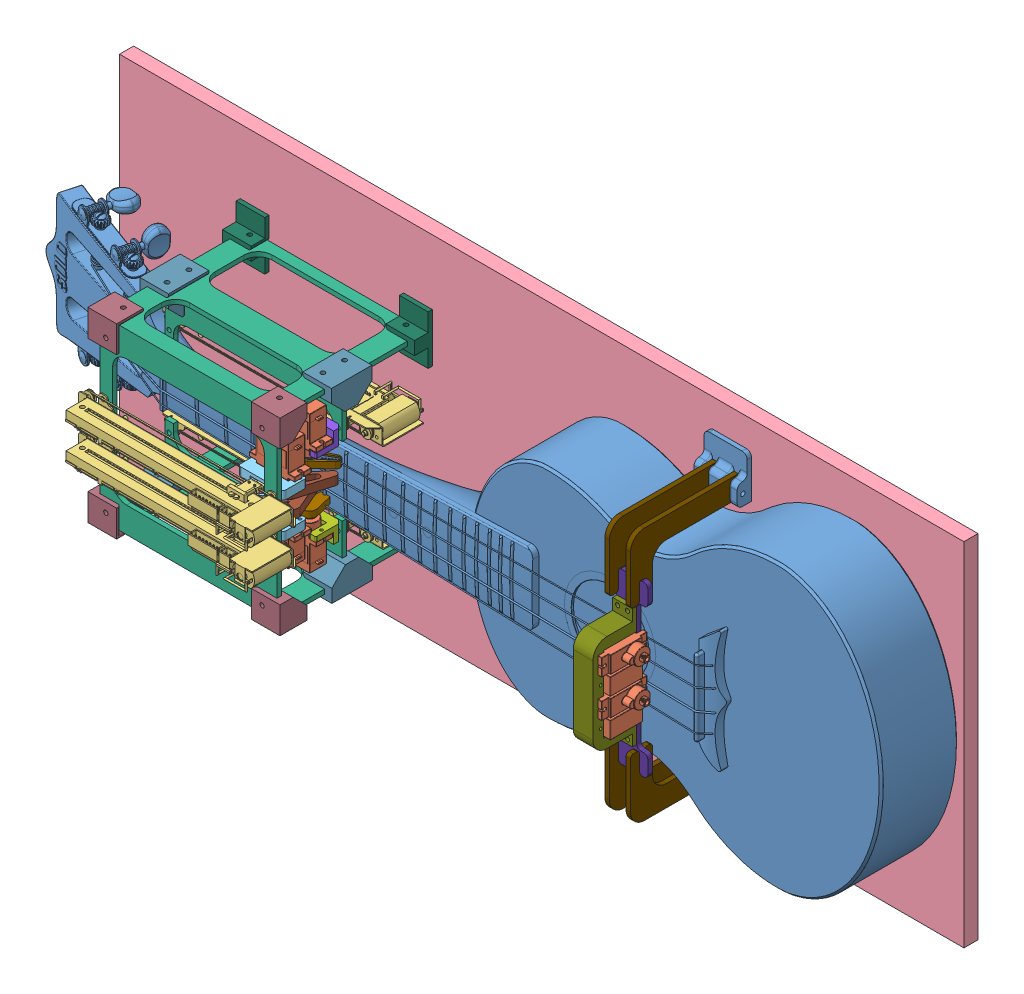
SolidWorks assembly GeneralAssembly, configuration Default. Lengths in mm.
Overall size (657.31 250 152.6).
52 component instances, 19 part files, 78 mates.
Components (placement in the parent):
- UKULELE-1: UKULELE [默认] at (479.369 -10.1459 0) size (657.31 214.72 74.19)
- Servo-MG90S-1: Servo-MG90S [Default] at (231.094 -48.7459 87.411) size (32.2 32.5 12.4)
- Servo-MG90S-2: Servo-MG90S [Default] at (231.094 28.4541 87.411) x (1 0 0) z (0 0 -1) size (32.2 32.5 12.4)
- Servo-MG90S-3: Servo-MG90S [Default] at (231.094 38.8541 72.089) x (1 0 0) z (0 0 -1) size (32.2 32.5 12.4)
- Servo-MG90S-4: Servo-MG90S [Default] at (231.094 -59.1459 72.089) size (32.2 32.5 12.4)
- Linear Actuator-1: Linear Actuator [Default] at (158.1164 97.3589 107.412) x (1 0 0) z (0 0 -1) size (152 13.58 46.19)
- Linear Actuator-2: Linear Actuator [Default] at (158.1164 72.1589 107.412) x (1 0 0) z (0 0 -1) size (152 13.58 46.19)
- Linear Actuator-3: Linear Actuator [Default] at (158.1164 -73.4506 52.588) size (152 13.58 46.19)
- Linear Actuator-4: Linear Actuator [Default] at (158.1164 -136.6506 52.588) size (152 13.58 46.19)
- BaseBoard-1: BaseBoard [Default] at (329.369 -10.1459 0) x (1 0 0) z (0 1 0) size (600 10 250)
- inner_servo_housing_EM_v2-1: inner_servo_housing_EM_v2 [Default] at (231.094 -22.7459 92.945) x (-1 0 0) z (0 1 0) size (32.2 17.07 6)
- inner_servo_housing_EM_v2-2: inner_servo_housing_EM_v2 [Default] at (231.094 2.4541 92.945) x (-1 0 0) z (0 1 0) size (32.2 17.07 6)
- Linear_Actuator_Housing_Sharon_V2-1: Linear_Actuator_Housing_Sharon_V2 [Default] at (246.369 -45.1459 8.5705) x (-1 0 0) z (0 1 0) size (126 105 126.35)
- bottom housing_Alice_V2-1: bottom housing_Alice_V2 [Default] at (230.83 -48.4167 63.7413) size (32.84 10.97 18.77)
- bottom housing_Alice_V2_right-1: bottom housing_Alice_V2_right [Default] at (230.83 -0.5567 63.7413) size (32.84 10.97 18.77)
- OuterFingerASM_Steven-1: OuterFingerASM_Steven [Default] at (243.2227 7.1953 66.202) x (0.575314 0 0.817933) z (0 -1 0) size (10 21.51 6.19)
  - OuterFinger_Steven-1: OuterFinger_Steven [Default] at (0.8965 2.1336 1.7571) size (10 21.51 4.5)
  - Servo Arm HXT900 Micro-1: Servo Arm HXT900 Micro [Default] at (6.3561 8.5439 5.0741) x (1 -0.000552 0) z (0 0 1) size (7.14 19.41 4.19)
- OuterFingerASM_Steven-2: OuterFingerASM_Steven [Default] at (236.3668 -27.487 63.0351) x (-0.995737 0 0.092235) z (0 1 0) size (10 21.51 6.19)
  - OuterFinger_Steven-1: OuterFinger_Steven [Default] at (0.8965 2.1336 1.7571) size (10 21.51 4.5)
  - Servo Arm HXT900 Micro-1: Servo Arm HXT900 Micro [Default] at (6.3561 8.5439 5.0741) x (1 -0.000552 0) z (0 0 1) size (7.14 19.41 4.19)
- InnerFinger_Anju_Assembly-1: InnerFinger_Anju_Assembly [Default] at (240.101 -41.1458 59.501) x (-0.979913 0 0.199427) z (0 1 0) size (15 33.85 6.3)
  - InnerFingerAnjuFinal-1: InnerFingerAnjuFinal [Default] at (9.2475 26.6001 21.6999) size (15 33.85 6)
  - Inner_Servo_Horn-1: Inner_Servo_Horn [Défaut] at (9.2475 26.6001 26.3999) x (1 0 0) z (0 0 -1) size (7.5 21 5)
- InnerFinger_Anju_Assembly-2: InnerFinger_Anju_Assembly [Default] at (240.7453 20.854 59.5953) x (0.881623 0 0.471955) z (0 -1 0) size (15 33.85 6.3)
  - InnerFingerAnjuFinal-1: InnerFingerAnjuFinal [Default] at (9.2475 26.6001 21.6999) size (15 33.85 6)
  - Inner_Servo_Horn-1: Inner_Servo_Horn [Défaut] at (9.2475 26.6001 26.3999) x (1 0 0) z (0 0 -1) size (7.5 21 5)
- ShelfCorner-1: ShelfCorner [Default] at (115.3004 49.7448 101.8991) size (20.4 19.05 19.05)
- ShelfMiddle-1: ShelfMiddle [Default] at (115.3009 49.7468 58.5983) x (1 0 0) z (0 1 0) size (20.4 28.74 19.05)
- ShelfBase-1: ShelfBase [Default] at (115.3075 52.9974 -0.0404) x (1 0 0) z (0 -1 0) size (20.4 12.75 34.86)
- PluckingServoHousing_Elinora-1: PluckingServoHousing_Elinora [Default] at (451.8619 -16.8459 85.2375) x (0 0 -1) z (0 -1 0) size (104.71 42 210.81)
  - Servo-MG90S-1: Servo-MG90S [Default] at origin size (32.2 32.5 12.4)
  - Servo-MG90S-2: Servo-MG90S [Default] at (0 23 13.4) x (1 0 0) z (0 0 -1) size (32.2 32.5 12.4)
  - Servo-MG90S-3: Servo-MG90S [Default] at (0 0 -26.8) size (32.2 32.5 12.4)
  - Servo-MG90S-4: Servo-MG90S [Default] at (0 23 -13.4) x (1 0 0) z (0 0 -1) size (32.2 32.5 12.4)
  - PluckingServoHolder_Elinora-2: PluckingServoHolder_Elinora [Default] at (-11.85 11.5 -6.7) x (0 1 0) z (0 0 1) size (14 31 85)
  - PluckingServoSupport-1: PluckingServoSupport [Default] at (11.65 11.5 -6.7) x (0 -1 0) z (0 0 1) size (30 3.17 120)
  - PluckingSupportLeg-1: PluckingSupportLeg [Default] at (5.2375 17.4125 38.3) x (0 0 -1) z (0 1 0) size (45 80 3.17)
  - PluckingSupportLeg-2: PluckingSupportLeg [Default] at (5.2375 20.5875 -51.7) x (0 0 1) z (0 -1 0) size (45 80 3.17)
  - PluckingSupportBase-1: PluckingSupportBase [Default] at (85.2817 -3.6182 68.3889) x (0 1 0) z (0 0 1) size (30.6 10.2 30.6)
  - PluckingSupportLeg-3: PluckingSupportLeg [Default] at (5.2375 2.4125 38.3) x (0 0 -1) z (0 1 0) size (45 80 3.17)
  - PluckingSupportLeg-4: PluckingSupportLeg [Default] at (5.2375 5.5875 -51.7) x (0 0 1) z (0 -1 0) size (45 80 3.17)
  - PluckingSupportBase-2: PluckingSupportBase [Default] at (84.825 26.6182 -81.7) x (0 -1 0) z (0 0 -1) size (30.6 10.2 30.6)
- ShelfBase-2: ShelfBase [Default] at (251.4305 49.8224 -0.0404) x (-1 0 0) z (0 1 0) size (20.4 12.75 34.86)
- ShelfCorner-2: ShelfCorner [Default] at (251.4376 49.7448 101.8991) x (-1 0 0) z (0 1 0) size (20.4 19.05 19.05)
- ShelfMiddle-2: ShelfMiddle [Default] at (251.4371 49.7468 55.7267) x (-1 0 0) z (0 1 0) size (20.4 28.74 19.05)
- ShelfBase-3: ShelfBase [Default] at (251.4305 -73.2891 -0.0404) x (-1 0 0) z (0 1 0) size (20.4 12.75 34.86)
- ShelfMiddle-3: ShelfMiddle [Default] at (251.4371 -70.0385 58.5983) x (-1 0 0) z (0 -1 0) size (20.4 28.74 19.05)
- ShelfCorner-3: ShelfCorner [Default] at (251.4376 -71.5006 101.8991) x (-1 0 0) z (0 0 1) size (20.4 19.05 19.05)
- ShelfMiddle-4: ShelfMiddle [Default] at (115.3009 -70.0385 55.7267) x (1 0 0) z (0 -1 0) size (20.4 28.74 19.05)
- ShelfCorner-4: ShelfCorner [Default] at (115.3004 -70.0365 101.8991) x (1 0 0) z (0 -1 0) size (20.4 19.05 19.05)
- ShelfBase-4: ShelfBase [Default] at (115.3075 -70.1141 -0.0404) x (1 0 0) z (0 -1 0) size (20.4 12.75 34.86)
Mates (geometry in assembly coordinates):
- Coincident2: coincident aligned: plane of Linear Actuator-1 through (119.369 4.9541 113.1) normal (-1 0 0); plane of Linear Actuator-2 through (119.369 -20.2459 113.1) normal (-1 0 0)
- Coincident3: coincident aligned: plane of Linear Actuator-2 through (119.369 -20.2459 113.1) normal (-1 0 0); plane of Linear Actuator-4 through (119.369 -44.2459 46.9) normal (-1 0 0)
- Coincident4: coincident aligned: plane of Linear Actuator-1 through (119.369 4.9541 113.1) normal (-1 0 0); plane of Linear Actuator-3 through (119.369 18.9541 46.9) normal (-1 0 0)
- Coincident8: coincident: plane of assembly through (0 0 0) normal (0 0 1); plane of UKULELE-1 through (494.4759 -89.9117 0) normal (0 0 -1); plane of assembly
- Distance5: distance = 215 mm aligned: plane of UKULELE-1 through (479.369 -10.1459 0) normal (1 0 0); plane of Linear Actuator-4 through (264.369 -35.7459 47.7) normal (1 0 0)
- Distance6: distance = 105 mm aligned: plane of Linear Actuator-2 through (112.369 -28.7459 105) normal (0 0 -1); plane of UKULELE-1 through (494.4759 -89.9117 0) normal (0 0 -1)
- Coincident10: coincident aligned: plane of Linear Actuator-1 through (237.989 8.1241 139.511) normal (0 0 1); plane of Linear Actuator-2 through (237.989 -17.0759 139.511) normal (0 0 1)
- Coincident11: coincident aligned: plane of Servo-MG90S-1 through (242.594 -30.2459 93.411) normal (1 0 0); plane of Servo-MG90S-3 through (242.594 20.3541 66.089) normal (1 0 0)
- Coincident13: coincident aligned: plane of Linear Actuator-3 through (112.369 27.4541 55) normal (0 0 1); plane of Linear Actuator-4 through (112.369 -35.7459 55) normal (0 0 1)
- Distance8: distance = 12 mm aligned: plane of Linear Actuator-2 through (233.344 -22.1459 105.611) normal (0 1 0); plane of UKULELE-1 through (479.369 -10.1459 0) normal (0 1 0)
- Distance9: distance = 31 mm aligned: plane of Linear Actuator-4 through (233.344 -41.1459 63.589) normal (0 1 0); plane of UKULELE-1 through (479.369 -10.1459 0) normal (0 1 0)
- Distance11: distance = 12 mm anti-aligned: plane of Linear Actuator-1 through (233.344 1.8541 96.411) normal (0 -1 0); plane of UKULELE-1 through (479.369 -10.1459 0) normal (0 1 0)
- Distance13: distance = 31 mm anti-aligned: plane of Linear Actuator-3 through (233.344 20.8541 54.389) normal (0 -1 0); plane of UKULELE-1 through (479.369 -10.1459 0) normal (0 1 0)
- Distance14: distance = 20 mm aligned: plane of Servo-MG90S-4 through (236.344 -30.1459 72.089) normal (0 1 0); plane of UKULELE-1 through (479.369 -10.1459 0) normal (0 1 0)
- Distance15: distance = 20 mm anti-aligned: plane of Servo-MG90S-3 through (236.344 9.8541 72.089) normal (0 -1 0); plane of UKULELE-1 through (479.369 -10.1459 0) normal (0 1 0)
- Coincident24: coincident aligned: plane of Servo-MG90S-1 through (231.094 -48.7459 93.611) normal (0 0 1); plane of Servo-MG90S-2 through (231.094 28.4541 93.611) normal (0 0 1)
- Coincident25: coincident aligned: plane of Servo-MG90S-1 through (242.594 -30.2459 93.411) normal (1 0 0); plane of Servo-MG90S-2 through (242.594 9.9541 81.411) normal (1 0 0)
- Coincident26: coincident aligned: plane of Servo-MG90S-3 through (242.594 20.3541 66.089) normal (1 0 0); plane of Servo-MG90S-4 through (242.594 -40.6459 78.089) normal (1 0 0)
- Coincident27: coincident aligned: plane of Servo-MG90S-3 through (231.094 38.8541 78.289) normal (0 0 1); plane of Servo-MG90S-4 through (231.094 -59.1459 78.289) normal (0 0 1)
- Distance18: distance = 0 mm aligned: plane of Servo-MG90S-4 through (242.594 -40.6459 78.089) normal (1 0 0); plane of Linear Actuator-4 through (242.594 -44.2943 50.2875) normal (1 0 0)
- Distance20: distance = 55 mm aligned: plane of Linear Actuator-4 through (112.369 -35.7459 55) normal (0 0 1); plane of UKULELE-1 through (479.369 -10.1459 0) normal (0 0 1)
- Distance21: distance = 2.5 mm anti-aligned: plane of Servo-MG90S-4 through (219.594 -40.6459 66.089) normal (0 0 -1); plane of Linear Actuator-4 through (233.344 -42.3459 63.589) normal (0 0 1)
- Distance22: distance = 15 mm aligned: plane of Servo-MG90S-1 through (219.594 -30.2459 81.411) normal (0 0 -1); plane of Linear Actuator-2 through (233.344 -22.1459 96.411) normal (0 0 -1)
- Coincident33: coincident anti-aligned: plane of UKULELE-1 through (494.4759 -89.9117 0) normal (0 0 -1); plane of BaseBoard-1 through (329.369 -10.1459 0) normal (0 0 1)
- Coincident34: coincident aligned: plane of UKULELE-1 through (479.369 -10.1459 0) normal (0 1 0); plane of BaseBoard-1 through (329.369 -10.1459 0) normal (0 1 0)
- Distance23: distance = 150 mm aligned: plane of BaseBoard-1 through (329.369 -10.1459 0) normal (1 0 0); plane of UKULELE-1 through (479.369 -10.1459 0) normal (1 0 0)
- Coincident37: coincident anti-aligned: plane of Servo-MG90S-1 through (231.094 -25.7459 87.411) normal (0 1 0); plane of inner_servo_housing_EM_v2-1 through (231.094 -25.7459 92.945) normal (0 -1 0)
- Coincident40: coincident anti-aligned: plane of Servo-MG90S-2 through (231.094 5.4541 87.411) normal (0 -1 0); plane of inner_servo_housing_EM_v2-2 through (231.094 5.4541 92.945) normal (0 1 0)
- Width1: width anti-aligned: plane of Linear Actuator-2 through (233.344 -22.1459 105.611) normal (0 1 0); plane of inner_servo_housing_EM_v2-1 through (233.344 -23.3459 96.411) normal (0 -1 0); plane of Linear Actuator-2 through (243.194 -21.9709 96.479) normal (0 -1 0); plane of inner_servo_housing_EM_v2-1 through (243.194 -23.5209 96.479) normal (0 1 0)
- Width2: width aligned: plane of Linear Actuator-1 through (233.344 3.0541 105.611) normal (0 1 0); plane of inner_servo_housing_EM_v2-2 through (233.344 1.8541 96.411) normal (0 -1 0); plane of Linear Actuator-1 through (243.194 1.6791 96.479) normal (0 1 0); plane of inner_servo_housing_EM_v2-2 through (243.194 3.2291 96.479) normal (0 -1 0)
- Coincident45: coincident anti-aligned: plane of BaseBoard-1 through (329.369 -10.1459 0) normal (0 0 1); plane of Linear_Actuator_Housing_Sharon_V2-1 through (120.369 -45.1459 0) normal (0 0 -1)
- Concentric2: concentric anti-aligned: cylinder of Linear Actuator-3 through (243.369 21.4541 55) axis (0 0 -1) radius 1.5; cylinder of Linear_Actuator_Housing_Sharon_V2-1 through (243.369 21.4541 -115.8139) axis (0 0 1) radius 1.5
- Concentric4: concentric aligned: cylinder of Servo-MG90S-1 through (217.244 -48.7459 87.411) axis (0 1 0) radius 1; cylinder of inner_servo_housing_EM_v2-1 through (217.244 -25.7459 87.411) axis (0 1 0) radius 1
- Concentric5: concentric aligned: cylinder of Servo-MG90S-1 through (244.944 -48.7459 87.411) axis (0 1 0) radius 1; cylinder of inner_servo_housing_EM_v2-1 through (244.944 -25.7459 87.411) axis (0 1 0) radius 1
- Concentric6: concentric anti-aligned: cylinder of Servo-MG90S-2 through (244.944 28.4541 87.411) axis (0 -1 0) radius 1; cylinder of inner_servo_housing_EM_v2-2 through (244.944 -0.5459 87.411) axis (0 1 0) radius 1
- Concentric7: concentric anti-aligned: cylinder of Servo-MG90S-2 through (217.244 28.4541 87.411) axis (0 -1 0) radius 1; cylinder of inner_servo_housing_EM_v2-2 through (217.244 -0.5459 87.411) axis (0 1 0) radius 1
- Coincident49: coincident anti-aligned: plane of Servo-MG90S-4 through (231.094 -37.6459 72.089) normal (0 1 0); plane of bottom housing_Alice_V2-1 through (214.3848 -37.6459 65.7619) normal (0 -1 0)
- Concentric9: concentric aligned: cylinder of Servo-MG90S-4 through (244.944 -59.1459 72.089) axis (0 1 0) radius 1; cylinder of bottom housing_Alice_V2-1 through (244.944 -45.8059 72.089) axis (0 1 0) radius 1.02
- Parallel1: parallel aligned: plane of Servo-MG90S-4 through (231.094 -59.1459 78.289) normal (0 0 1); plane of bottom housing_Alice_V2-1 through (230.8068 -48.6109 65.7619) normal (0 0 1)
- Concentric13: concentric aligned: cylinder of Servo-MG90S-3 through (244.944 38.8541 72.089) axis (0 -1 0) radius 1; cylinder of bottom housing_Alice_V2_right-1 through (244.944 25.5141 72.089) axis (0 -1 0) radius 1.02
- Parallel4: parallel aligned: plane of Servo-MG90S-3 through (231.094 38.8541 78.289) normal (0 0 1); plane of bottom housing_Alice_V2_right-1 through (230.8068 28.3191 65.7619) normal (0 0 1)
- Coincident54: coincident anti-aligned: plane of Servo-MG90S-3 through (231.094 17.3541 72.089) normal (0 -1 0); plane of bottom housing_Alice_V2_right-1 through (214.3848 17.3541 65.7619) normal (0 1 0)
- Concentric14: concentric anti-aligned: cylinder of Servo-MG90S-3 through (236.344 8.8541 72.089) axis (0 -1 0) radius 1.25; cylinder of OuterFingerASM_Steven-1/OuterFinger_Steven-1 through (236.344 2.9631 72.089) axis (0 1 0) radius 5
- Coincident55: coincident anti-aligned: plane of Servo-MG90S-3 through (236.344 6.3541 72.089) normal (0 -1 0); plane of OuterFingerASM_Steven-1/Servo Arm HXT900 Micro-1 through (236.7245 6.3541 71.8194) normal (0 1 0)
- Concentric15: concentric anti-aligned: cylinder of Servo-MG90S-4 through (236.344 -29.1459 72.089) axis (0 1 0) radius 1.25; cylinder of OuterFingerASM_Steven-2/OuterFinger_Steven-1 through (236.344 -23.2549 72.089) axis (0 -1 0) radius 5
- Coincident56: coincident anti-aligned: plane of Servo-MG90S-4 through (236.344 -26.6459 72.089) normal (0 1 0); plane of OuterFingerASM_Steven-2/Servo Arm HXT900 Micro-1 through (236.3027 -26.6459 71.6246) normal (0 -1 0)
- Concentric17: concentric anti-aligned: cylinder of Servo-MG90S-1 through (236.344 -18.7459 87.411) axis (0 1 0) radius 1.25; cylinder of InnerFinger_Anju_Assembly-1/InnerFingerAnjuFinal-1 through (236.344 -13.4459 87.411) axis (0 -1 0) radius 7.5
- Coincident57: coincident anti-aligned: plane of Servo-MG90S-1 through (236.344 -16.2459 87.411) normal (0 1 0); plane of InnerFinger_Anju_Assembly-1/Inner_Servo_Horn-1 through (236.344 -16.2459 87.411) normal (0 -1 0)
- Concentric18: concentric anti-aligned: cylinder of Servo-MG90S-2 through (236.344 -1.5459 87.411) axis (0 -1 0) radius 1.25; cylinder of InnerFinger_Anju_Assembly-2/InnerFingerAnjuFinal-1 through (236.344 -6.8459 87.411) axis (0 1 0) radius 7.5
- Coincident59: coincident anti-aligned: plane of Servo-MG90S-2 through (236.344 -4.0459 87.411) normal (0 -1 0); plane of InnerFinger_Anju_Assembly-2/Inner_Servo_Horn-1 through (236.344 -4.0459 87.411) normal (0 1 0)
- Concentric19: concentric aligned: cylinder of ShelfCorner-1 through (127.869 37.0406 95.825) axis (0 1 0) radius 1.53; cylinder of Linear_Actuator_Housing_Sharon_V2-1 through (127.869 -73.3209 95.825) axis (0 1 0) radius 1.5
- Parallel5: parallel aligned: plane of Linear_Actuator_Housing_Sharon_V2-1 through (120.369 -45.1459 105) normal (0 0 1); plane of ShelfCorner-1 through (135.519 56.0891 108.2435) normal (0 0 1)
- Concentric22: concentric aligned: cylinder of Linear_Actuator_Housing_Sharon_V2-1 through (127.869 -73.3209 64.75) axis (0 1 0) radius 1.5; cylinder of ShelfMiddle-1 through (127.869 37.0406 64.75) axis (0 1 0) radius 1.53
- Coincident63: coincident anti-aligned: plane of Linear_Actuator_Housing_Sharon_V2-1 through (246.369 53.0291 101.825) normal (0 1 0); plane of ShelfMiddle-1 through (120.219 53.0291 55.3915) normal (0 -1 0)
- Concentric23: concentric anti-aligned: cylinder of Linear_Actuator_Housing_Sharon_V2-1 through (127.869 -73.3209 6) axis (0 1 0) radius 1.5; cylinder of ShelfBase-1 through (127.869 68.8391 6) axis (0 -1 0) radius 1.53
- Coincident66: coincident anti-aligned: plane of UKULELE-1 through (479.369 -10.1459 0) normal (0 1 0); plane of Linear_Actuator_Housing_Sharon_V2-1 through (246.369 -10.1459 8.5705) normal (0 -1 0)
- Parallel10: parallel anti-aligned: plane of BaseBoard-1 through (329.369 -10.1459 0) normal (0 0 1); plane of ShelfBase-1 through (135.519 53.0291 -0.12) normal (0 0 -1)
- Coincident68: coincident anti-aligned: plane of Linear_Actuator_Housing_Sharon_V2-1 through (246.369 53.0291 101.825) normal (0 1 0); plane of ShelfBase-1 through (120.219 53.0291 12.63) normal (0 -1 0)
- Coincident69: coincident anti-aligned: plane of BaseBoard-1 through (329.369 -10.1459 0) normal (0 0 1); plane of PluckingServoHousing_Elinora-1/PluckingSupportLeg-1 through (472.4494 -55.1459 0) normal (0 0 -1)
- Coincident70: coincident anti-aligned: plane of UKULELE-1 through (479.369 -10.1459 0) normal (0 1 0); plane of PluckingServoHousing_Elinora-1/PluckingServoSupport-1 through (463.3619 -10.1459 73.5875) normal (0 -1 0)
- Concentric25: concentric aligned: cylinder of Linear_Actuator_Housing_Sharon_V2-1 through (238.869 -73.3209 6) axis (0 1 0) radius 1.5; cylinder of ShelfBase-2 through (238.869 33.9806 6) axis (0 1 0) radius 1.53
- Coincident72: coincident anti-aligned: plane of Linear_Actuator_Housing_Sharon_V2-1 through (246.369 53.0291 101.825) normal (0 1 0); plane of ShelfBase-2 through (246.519 53.0291 12.63) normal (0 -1 0)
- Parallel12: parallel aligned: plane of BaseBoard-1 through (329.369 -10.1459 0) normal (0 0 1); plane of ShelfBase-2 through (231.219 56.0891 2.94) normal (0 0 1)
- Coincident74: coincident anti-aligned: plane of Linear_Actuator_Housing_Sharon_V2-1 through (246.369 53.0291 101.825) normal (0 1 0); plane of ShelfMiddle-2 through (246.519 53.0291 58.9335) normal (0 -1 0)
- Concentric26: concentric aligned: cylinder of Linear_Actuator_Housing_Sharon_V2-1 through (238.869 -73.3209 49.575) axis (0 1 0) radius 1.5; cylinder of ShelfMiddle-2 through (238.869 37.0406 49.575) axis (0 1 0) radius 1.53
- Parallel13: parallel aligned: plane of BaseBoard-1 through (329.369 -10.1459 0) normal (0 0 1); plane of ShelfMiddle-2 through (231.219 56.0891 71.6835) normal (0 0 1)
- Concentric28: concentric aligned: cylinder of Linear_Actuator_Housing_Sharon_V2-1 through (238.869 -73.3209 95.825) axis (0 1 0) radius 1.5; cylinder of ShelfCorner-2 through (238.869 37.0406 95.825) axis (0 1 0) radius 1.53
- Coincident77: coincident anti-aligned: plane of Linear_Actuator_Housing_Sharon_V2-1 through (246.369 53.0291 101.825) normal (0 1 0); plane of ShelfCorner-2 through (246.519 53.0291 105.1835) normal (0 -1 0)
- Parallel15: parallel aligned: plane of Linear_Actuator_Housing_Sharon_V2-1 through (120.369 -45.1459 105) normal (0 0 1); plane of ShelfCorner-2 through (231.219 37.0406 108.2435) normal (0 0 1)
- Coincident79: coincident anti-aligned: plane of Linear_Actuator_Housing_Sharon_V2-1 through (246.369 53.0291 101.825) normal (0 1 0); plane of ShelfCorner-1 through (120.219 53.0291 89.195) normal (0 -1 0)
- Parallel16: parallel anti-aligned: plane of BaseBoard-1 through (329.369 -10.1459 0) normal (0 0 1); plane of ShelfMiddle-1 through (135.519 56.0891 42.6415) normal (0 0 -1)
- Coincident81: coincident aligned: plane of ShelfBase-2 through (251.619 49.7906 -0.12) normal (1 0 0); plane of ShelfBase-3 through (251.619 -73.3209 -0.12) normal (1 0 0)
- Coincident82: coincident aligned: plane of ShelfMiddle-2 through (251.619 49.7906 55.695) normal (1 0 0); plane of ShelfMiddle-3 through (251.619 -70.0824 58.63) normal (1 0 0)
- Coincident84: coincident aligned: plane of ShelfBase-1 through (115.119 53.0291 -0.12) normal (-1 0 0); plane of ShelfBase-4 through (115.119 -70.0824 -0.12) normal (-1 0 0)
- Coincident85: coincident aligned: plane of ShelfMiddle-1 through (115.119 49.7906 58.63) normal (-1 0 0); plane of ShelfMiddle-4 through (115.119 -70.0824 55.695) normal (-1 0 0)
- Coincident86: coincident aligned: plane of ShelfCorner-1 through (115.119 49.7906 101.945) normal (-1 0 0); plane of ShelfCorner-4 through (115.119 -70.0824 101.945) normal (-1 0 0)
- Coincident87: coincident aligned: plane of ShelfCorner-2 through (251.619 49.7906 101.945) normal (1 0 0); plane of ShelfCorner-3 through (251.619 -71.5465 101.945) normal (1 0 0)
- Coincident88: coincident aligned: plane of Linear Actuator-4 through (246.369 -36.5459 55) normal (1 0 0); plane of Linear_Actuator_Housing_Sharon_V2-1 through (246.369 -45.1459 8.5705) normal (1 0 0)
